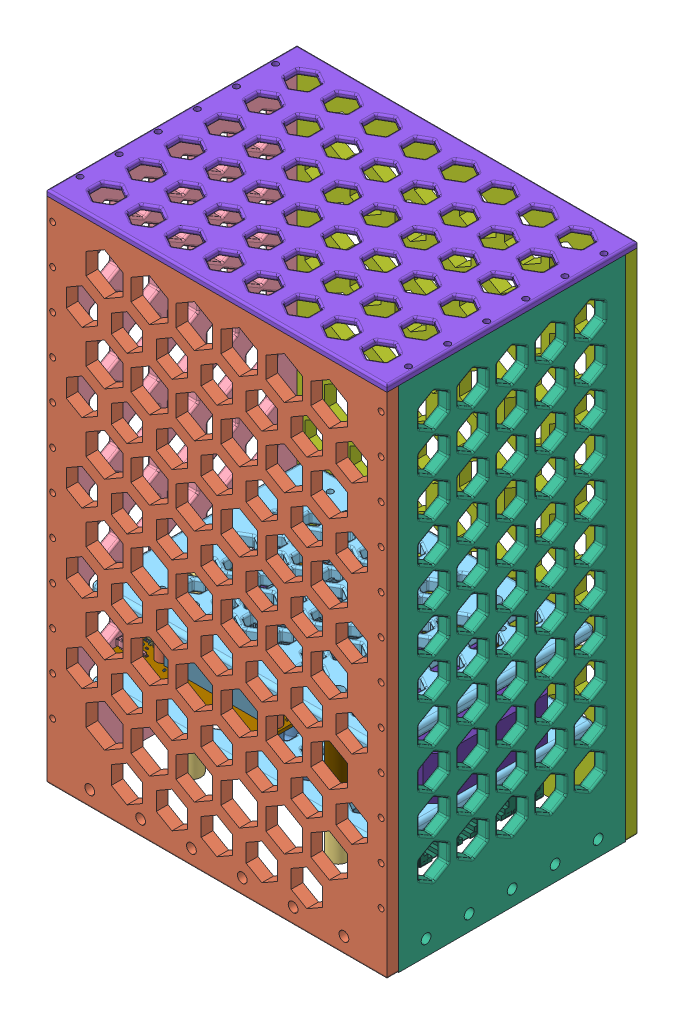
SolidWorks assembly upperbody, configuration 默认. Lengths in mm.
Overall size (174 266.08 128).
496 component instances, 112 part files, 71 mates.
Components (placement in the parent):
- battery-1: battery [默认] at (3.2915 206.5588 214.1011) x (-1 0 0) z (0 -1 0) size (140 115 140)
- imu-1: imu [默认] at (5.7743 27.9888 133.0371) x (0 0 -1) z (0 1 0) size (79.76 40 69.46)
- front-1: front [默认] at (4.5084 194.9888 220) size (174 260 6)
- M8螺柱-1: M8螺柱 [默认] at (42.5084 62.9888 122) size (10 25 10)
- M8螺柱-2: M8螺柱 [默认] at (42.5084 62.9888 202) x (0.721666 0 -0.692241) z (0.692241 0 0.721666) size (10 25 10)
- M8螺柱-3: M8螺柱 [默认] at (-32.4916 62.9888 122) x (0.928948 0 -0.370211) z (0.370211 0 0.928948) size (10 25 10)
- M8螺柱-4: M8螺柱 [默认] at (-32.4916 62.9888 202) x (0.697956 0 -0.71614) z (0.71614 0 0.697956) size (10 25 10)
- left-1: left [默认] at (-82.4916 204.9888 162) x (0 0 -1) z (1 0 0) size (116 260 6)
- ctrlbox-2: ctrlbox [默认] at (5.0084 87.9888 162) size (148 6 110)
- right-1: right [默认] at (91.5084 204.9888 162) x (0 0 1) z (-1 0 0) size (116 260 6)
- back-2: back [默认] at (4.5084 194.9888 98) size (174 260 6)
- top-1: top [默认] at (4.5084 304.9888 162) size (174 6.16 128)
- jetsonnano-1: jetsonnano [默认] at (-39.9804 116.3688 223.5192) x (0 0 1) z (0 1 0) size (100.18 80.53 31.78)
  - 675_13541_batuu_dev_kit_top_ass_asm.stp-1: 675_13541_batuu_dev_kit_top_ass_asm.stp [Default] at (-107.5192 -7.5112 -12.38) size (100.18 80.53 31.78)
    - 642-13541_BATUU_SYS_BOM_ASM.stp-1: 642-13541_BATUU_SYS_BOM_ASM.stp [Default] at origin size (100.18 80.53 21.55)
      - 600-13542-BASE-A02_ASM.stp-1: 600-13542-BASE-A02_ASM.stp [Default] at origin size (100.18 80.53 21.55)
        - 600-13542-BASE-A02.stp-1: 600-13542-BASE-A02.stp [Default] at origin size (100 79 1.57)
        - 064-0473-000_1.stp-1: 064-0473-000_1.stp [Default] at (2.055 -14.41 1.57) size (11.16 8.51 5.94)
        - LOGO_SILK_180_I560.stp-1: LOGO_SILK_180_I560.stp [Default] at (2.088 17.507 0) x (0 1 0) z (0 0 -1) size (14.3 1.27 0.05)
        - LOGO_SILK_POSTAL_ADDRESS.stp-1: LOGO_SILK_POSTAL_ADDRESS.stp [Default] at (3.985 7.597 0) x (0 1 0) z (0 0 -1) size (18.11 2.17 0.05)
        - LS_ICES_I0925X0040_CLASS_B.stp-1: LS_ICES_I0925X0040_CLASS_B.stp [Default] at (0.822 15.645 0) x (0 1 0) z (0 0 -1) size (17.94 1.42 0.03)
        - LOGO_SILK_P3542.stp-1: LOGO_SILK_P3542.stp [Default] at (-1.446 36.987 0) x (0 1 0) z (0 0 -1) size (6.18 1.16 0.01)
        - LOGO_SILK_ROHS_I0300X0153.stp-1: LOGO_SILK_ROHS_I0300X0153.stp [Default] at (0.509 33.093 0) x (0 1 0) z (0 0 -1) size (7.55 3.9 0.05)
        - LOGO_SILK_NVIDIA_I0400X0240.stp-1: LOGO_SILK_NVIDIA_I0400X0240.stp [Default] at (10.037 11.31 0) x (0 1 0) z (0 0 -1) size (7.63 5.72 0.1)
        - 115-1921-000_3.stp-1: 115-1921-000_3.stp [Default] at (71 38 1.57) x (0 -1 0) z (0 0 1) size (5 4 1.01)
        - 115-1921-000_3.stp-2: 115-1921-000_3.stp [Default] at (71 46.5 1.57) x (0 -1 0) z (0 0 1) size (5 4 1.01)
        - 115-1921-000_3.stp-3: 115-1921-000_3.stp [Default] at (71 29.5 1.57) x (0 -1 0) z (0 0 1) size (5 4 1.01)
        - LS_CTUVUS_0500X0500_SIMPLE.stp-1: LS_CTUVUS_0500X0500_SIMPLE.stp [Default] at (49.36 31.942 0) x (-1 0 0) z (0 0 -1) size (5.04 5.01 0.05)
        - LOGO_SILK_UKRAINE_0500X0500.stp-1: LOGO_SILK_UKRAINE_0500X0500.stp [Default] at (41 32.494 0) x (-1 0 0) z (0 0 -1) size (4.37 5.01 0.05)
        - LOGO_SILK_SAA_1206X0540.stp-1: LOGO_SILK_SAA_1206X0540.stp [Default] at (44.276 41.966 0) x (-1 0 0) z (0 0 -1) size (12.08 8.03 0.06)
        - 064-0476-000_1.stp-1: 064-0476-000_1.stp [Default] at (55.6 -9.269 1.57) size (14.86 17.99 18.47)
        - 064-0472-000_1.stp-1: 064-0472-000_1.stp [Default] at (88 -14.3 1.57) size (8.8 6.34 3.46)
        - 0402_SHUNT_NO.stp-1: 0402_SHUNT_NO.stp [Default] at (57.444 37.6 1.57) size (1.51 0.51 0.03)
        - 0402_SHUNT_NO.stp-2: 0402_SHUNT_NO.stp [Default] at (55.15 36.025 1.57) x (0 1 0) z (0 0 1) size (1.51 0.51 0.03)
        - 0402_SHUNT_NO.stp-3: 0402_SHUNT_NO.stp [Default] at (55.15 33.762 1.57) x (0 -1 0) z (0 0 1) size (1.51 0.51 0.03)
        - 0402_SHORT.stp-1: 0402_SHORT.stp [Default] at (57.6 38.53 1.57) size (1.51 0.51 1)
        - 0402_SHORT.stp-2: 0402_SHORT.stp [Default] at (53.708 35.675 1.57) x (-1 0 0) z (0 0 1) size (1.51 0.51 1)
        - 0402_SHORT.stp-3: 0402_SHORT.stp [Default] at (53.708 34.112 1.57) x (-1 0 0) z (0 0 1) size (1.51 0.51 1)
        - 0402_SHORT.stp-4: 0402_SHORT.stp [Default] at (60.9 37.1 1.57) x (0 -1 0) z (0 0 1) size (1.51 0.51 1)
        - 064-0474-000_1.stp-1: 064-0474-000_1.stp [Default] at (38.6 -9.759 1.57) size (14.81 17.11 9.91)
        - 085-0347-000_1.stp-1: 085-0347-000_1.stp [Default] at (31.173 31.804 1.57) x (0 -1 0) z (0 0 1) size (3.6 2.9 0.81)
        - 115-2844-000_1.stp-1: 115-2844-000_1.stp [Default] at (39.89 33.254 1.57) x (0 1 0) z (0 0 1) size (5.01 7.06 1.76)
        - 074-0259-000_1.stp-1: 074-0259-000_1.stp [Default] at (19.751 -12.06 1.57) x (0 1 0) z (0 0 1) size (13.02 16.16 8.1)
        - 106-0078-000_1.stp-1: 106-0078-000_1.stp [Default] at (4.864 -6.11 1.57) size (6.08 4.44 1.61)
        - LOGO_SILK_EAC_050X050.stp-1: LOGO_SILK_EAC_050X050.stp [Default] at (28.157 35.506 0) x (-1 0 0) z (0 0 -1) size (5 5 0.05)
        - LOGO_LABEL_PPID_0180X0050.stp-1: LOGO_LABEL_PPID_0180X0050.stp [Default] at (49.45 19.35 0) x (-1 0 0) z (0 0 -1) size (18 5 0.15)
        - 074-0221-000_3.stp-1: 074-0221-000_3.stp [Default] at (86 29 1.57) x (0 1 0) z (0 0 1) size (51.01 5.29 12.01)
        - 080-1656-000_3.stp-1: 080-1656-000_3.stp [Default] at (44 16.6 1.57) x (-1 0 0) z (0 0 1) size (77.5 26.11 9.91)
        - 080-1669-000_2.stp-1: 080-1669-000_2.stp [Default] at (0.2 29 1.57) x (0 -1 0) z (0 0 1) size (22.61 5.4 8.01)
        - 064-0400-000_1.stp-1: 064-0400-000_1.stp [Default] at (67.5 7.785 1.57) size (10.42 6.06 13.91)
        - 220-0146-000_2.stp-1: 220-0146-000_2.stp [Default] at (59.96 55.2 0) x (-1 0 0) z (0 0 -1) size (19.53 12.33 3.44)
        - 074-0239-000_1.stp-1: 074-0239-000_1.stp [Default] at (31.71 54.5 1.57) x (-1 0 0) z (0 0 1) size (30.59 10.8 5.76)
        - 0603_H100.stp-1: 0603_H100.stp [Default] at (34.617 32.966 1.57) x (0 1 0) z (0 0 1) size (1.81 1.01 1.01)
        - 0603_H100.stp-2: 0603_H100.stp [Default] at (33.893 7.175 1.57) x (-1 0 0) z (0 0 1) size (1.81 1.01 1.01)
        - 0603_H100.stp-3: 0603_H100.stp [Default] at (20.2 35 1.57) x (-1 0 0) z (0 0 1) size (1.81 1.01 1.01)
        - 0603_H100.stp-4: 0603_H100.stp [Default] at (20.2 33.55 1.57) x (-1 0 0) z (0 0 1) size (1.81 1.01 1.01)
        - 0603_H100.stp-5: 0603_H100.stp [Default] at (13.895 41.85 1.57) x (-1 0 0) z (0 0 1) size (1.81 1.01 1.01)
        - 0603_H100.stp-6: 0603_H100.stp [Default] at (7.3 3.117 1.57) size (1.81 1.01 1.01)
        - 0603_H100.stp-7: 0603_H100.stp [Default] at (11.03 6.374 1.57) x (0 1 0) z (0 0 1) size (1.81 1.01 1.01)
        - 0603_H060.stp-1: 0603_H060.stp [Default] at (63.195 1.13 1.57) size (1.81 1.02 0.61)
        - 0603_H060.stp-2: 0603_H060.stp [Default] at (82.541 -6.821 1.57) x (-1 0 0) z (0 0 1) size (1.81 1.02 0.61)
        - 0603_H060.stp-3: 0603_H060.stp [Default] at (82.541 -9.047 1.57) x (-1 0 0) z (0 0 1) size (1.81 1.02 0.61)
        - FID_40_80SM.stp-1: FID_40_80SM.stp [Default] at (80.7 59.5 1.57) size (2.29 2.29 0.05)
        - FID_40_80SM.stp-2: FID_40_80SM.stp [Default] at (7.943 54.544 1.57) size (2.29 2.29 0.05)
        - FID_40_80SM.stp-3: FID_40_80SM.stp [Default] at (93.132 -0.325 1.57) size (2.29 2.29 0.05)
        - FID_40_80SM.stp-4: FID_40_80SM.stp [Default] at (9.9 22.4 0) x (-1 0 0) z (0 0 -1) size (2.29 2.29 0.05)
        - FID_40_80SM.stp-5: FID_40_80SM.stp [Default] at (80.7 59.5 0) x (-1 0 0) z (0 0 -1) size (2.29 2.29 0.05)
        - FID_40_80SM.stp-6: FID_40_80SM.stp [Default] at (3.95 -6.475 0) x (-1 0 0) z (0 0 -1) size (2.29 2.29 0.05)
        - LOGO_SILK_ROHS_D050_CHINA.stp-1: LOGO_SILK_ROHS_D050_CHINA.stp [Default] at (35.305 32.341 0) x (-1 0 0) z (0 0 -1) size (5.62 4.99 0.05)
        - LOGO_SILK_WEEE_0485X0683.stp-1: LOGO_SILK_WEEE_0485X0683.stp [Default] at (28.183 29 0) x (-1 0 0) z (0 0 -1) size (4.85 6.82 0.05)
        - LOGO_SILK_VCCI_I0300X0225.stp-1: LOGO_SILK_VCCI_I0300X0225.stp [Default] at (55.897 33.25 0) x (-1 0 0) z (0 0 -1) size (8.32 6.14 0.05)
        - LOGO_SILK_RCM_040X030.stp-1: LOGO_SILK_RCM_040X030.stp [Default] at (57.832 27.06 0) x (-1 0 0) z (0 0 -1) size (4.05 3 0.05)
        - LOGO_SILK_BSMI_I0138H.stp-1: LOGO_SILK_BSMI_I0138H.stp [Default] at (52.892 27.23 0) x (-1 0 0) z (0 0 -1) size (8.8 3.76 0.05)
        - LOGO_SILK_HF_I0185X0120.stp-1: LOGO_SILK_HF_I0185X0120.stp [Default] at (37.6 25.2 0) x (-1 0 0) z (0 0 -1) size (4.83 3.17 0.07)
        - 090-0243-000_1.stp-1: 090-0243-000_1.stp [Default] at (88.606 -9.875 1.57) size (1.41 0.71 0.46)
        - 090-0243-000_1.stp-2: 090-0243-000_1.stp [Default] at (86.685 -9.875 1.57) x (-1 0 0) z (0 0 1) size (1.41 0.71 0.46)
        - 090-0243-000_1.stp-3: 090-0243-000_1.stp [Default] at (43.22 0.665 1.57) size (1.41 0.71 0.46)
        - 090-0243-000_1.stp-4: 090-0243-000_1.stp [Default] at (41.15 0.665 1.57) x (-1 0 0) z (0 0 1) size (1.41 0.71 0.46)
        - 090-0243-000_1.stp-5: 090-0243-000_1.stp [Default] at (11.85 27.85 1.57) size (1.41 0.71 0.46)
        - 090-0243-000_1.stp-6: 090-0243-000_1.stp [Default] at (12.358 6.374 1.57) x (0 1 0) z (0 0 1) size (1.41 0.71 0.46)
        - 090-0243-000_1.stp-7: 090-0243-000_1.stp [Default] at (19.35 -1.5 1.57) size (1.41 0.71 0.46)
        - 090-0243-000_1.stp-8: 090-0243-000_1.stp [Default] at (17.358 -1.5 1.57) size (1.41 0.71 0.46)
        - 090-0243-000_1.stp-9: 090-0243-000_1.stp [Default] at (15.308 -1.5 1.57) x (-1 0 0) z (0 0 1) size (1.41 0.71 0.46)
        - 090-0243-000_1.stp-10: 090-0243-000_1.stp [Default] at (13.064 -4.054 1.57) x (-1 0 0) z (0 0 1) size (1.41 0.71 0.46)
        - 090-0243-000_1.stp-11: 090-0243-000_1.stp [Default] at (3.491 18.432 1.57) x (0 -1 0) z (0 0 1) size (1.41 0.71 0.46)
        - 090-0243-000_1.stp-12: 090-0243-000_1.stp [Default] at (5.016 18.432 1.57) x (0 -1 0) z (0 0 1) size (1.41 0.71 0.46)
        - 090-0243-000_1.stp-13: 090-0243-000_1.stp [Default] at (11.85 23.6 1.57) size (1.41 0.71 0.46)
        - 090-0243-000_1.stp-14: 090-0243-000_1.stp [Default] at (11.85 25.25 1.57) size (1.41 0.71 0.46)
        - 090-0243-000_1.stp-15: 090-0243-000_1.stp [Default] at (11.85 26.5 1.57) size (1.41 0.71 0.46)
        - 091-0023-000_1.stp-1: 091-0023-000_1.stp [Default] at (17.098 5.642 1.57) size (2.21 2.51 1.11)
        - 115-2747-000_1.stp-1: 115-2747-000_1.stp [Default] at (11.957 32.276 1.57) x (0 1 0) z (0 0 1) size (2.21 2.88 1.11)
        - 115-0742-000_2.stp-1: 115-0742-000_2.stp [Default] at (5.725 44.6 1.57) size (2.21 2.88 1.11)
        - 115-1821-000_1.stp-1: 115-1821-000_1.stp [Default] at (12.1 48.825 1.57) x (0 -1 0) z (0 0 1) size (2.21 2.88 1.11)
        - 115-1821-000_1.stp-2: 115-1821-000_1.stp [Default] at (8.55 44.6 1.57) x (-1 0 0) z (0 0 1) size (2.21 2.88 1.11)
        - 115-0138-000_1.stp-1: 115-0138-000_1.stp [Default] at (59.536 5.825 1.57) x (-1 0 0) z (0 0 1) size (2.21 2.88 1.11)
        - 115-0742-000_2.stp-2: 115-0742-000_2.stp [Default] at (11.3 44.6 1.57) x (-1 0 0) z (0 0 1) size (2.21 2.88 1.11)
        - 315-1048-000_1.stp-1: 315-1048-000_1.stp [Default] at (7.151 6.724 1.57) x (0 1 0) z (0 0 1) size (3.11 3.58 1.46)
        - 315-1014-000_1.stp-1: 315-1014-000_1.stp [Default] at (36.977 7.376 1.57) size (3.11 3.58 1.46)
        - 315-0620-000_1.stp-1: 315-0620-000_1.stp [Default] at (53.589 41.71 1.57) x (0 -1 0) z (0 0 1) size (3.11 3.58 1.11)
        - LOGO_SILK_CE_I0175X0160.stp-1: LOGO_SILK_CE_I0175X0160.stp [Default] at (41.179 26.706 0) x (-1 0 0) z (0 0 -1) size (4.55 3.29 0.05)
        - 090-0231-000_1.stp-1: 090-0231-000_1.stp [Default] at (56.393 1.13 1.57) x (-1 0 0) z (0 0 1) size (2.61 1.55 0.56)
        - 090-0231-000_1.stp-2: 090-0231-000_1.stp [Default] at (25.625 -1.95 1.57) x (-1 0 0) z (0 0 1) size (2.61 1.55 0.56)
        - 090-0231-000_1.stp-3: 090-0231-000_1.stp [Default] at (21.95 -1.95 1.57) size (2.61 1.55 0.56)
        - 090-0231-000_1.stp-4: 090-0231-000_1.stp [Default] at (38.6 0.417 1.57) size (2.61 1.55 0.56)
        - 0402_H040.stp-1: 0402_H040.stp [Default] at (61.419 6.962 1.57) x (0 1 0) z (0 0 1) size (1.2 0.61 0.41)
        - 0402_H060.stp-1: 0402_H060.stp [Default] at (3.646 48.98 1.57) x (0 -1 0) z (0 0 1) size (1.11 0.61 0.61)
        - 0402_H060.stp-2: 0402_H060.stp [Default] at (82.141 -12.349 1.57) x (-1 0 0) z (0 0 1) size (1.11 0.61 0.61)
        - 0402_H060.stp-3: 0402_H060.stp [Default] at (85.011 -10.767 1.57) x (-1 0 0) z (0 0 1) size (1.11 0.61 0.61)
        - 0402_H040.stp-2: 0402_H040.stp [Default] at (57.017 6.2 1.57) x (0 1 0) z (0 0 1) size (1.2 0.61 0.41)
        - 0402_H060.stp-4: 0402_H060.stp [Default] at (50.674 42.15 1.57) x (0 -1 0) z (0 0 1) size (1.11 0.61 0.61)
        - 0402_H060.stp-5: 0402_H060.stp [Default] at (56.489 42.038 1.57) x (0 -1 0) z (0 0 1) size (1.11 0.61 0.61)
        - 0402_H060.stp-6: 0402_H060.stp [Default] at (9.475 49.55 1.57) x (0 1 0) z (0 0 1) size (1.11 0.61 0.61)
        - 0402_H040.stp-3: 0402_H040.stp [Default] at (35.099 35.617 1.57) size (1.2 0.61 0.41)
        - 0402_H040.stp-4: 0402_H040.stp [Default] at (37.596 37.35 1.57) x (-1 0 0) z (0 0 1) size (1.2 0.61 0.41)
        - 0402_H040.stp-5: 0402_H040.stp [Default] at (85.653 -8.168 1.57) x (0 1 0) z (0 0 1) size (1.2 0.61 0.41)
        - 0402_H060.stp-7: 0402_H060.stp [Default] at (33.493 30.304 1.57) x (0 1 0) z (0 0 1) size (1.11 0.61 0.61)
        - 0402_H060.stp-8: 0402_H060.stp [Default] at (33.493 32.251 1.57) x (0 1 0) z (0 0 1) size (1.11 0.61 0.61)
        - 0402_H060.stp-9: 0402_H060.stp [Default] at (35.099 34.667 1.57) x (-1 0 0) z (0 0 1) size (1.11 0.61 0.61)
        - 0402_H060.stp-10: 0402_H060.stp [Default] at (33.45 36.567 1.57) x (-1 0 0) z (0 0 1) size (1.11 0.61 0.61)
        - 0402_H060.stp-11: 0402_H060.stp [Default] at (33.45 35.617 1.57) x (-1 0 0) z (0 0 1) size (1.11 0.61 0.61)
        - 0402_H040.stp-6: 0402_H040.stp [Default] at (14.693 -3.538 1.57) x (0 -1 0) z (0 0 1) size (1.2 0.61 0.41)
        - 0402_H060.stp-12: 0402_H060.stp [Default] at (50.945 26.269 1.57) size (1.11 0.61 0.61)
        - 0402_H060.stp-13: 0402_H060.stp [Default] at (53.281 0.53 1.57) size (1.11 0.61 0.61)
        - 0402_H060.stp-14: 0402_H060.stp [Default] at (30.208 -2.121 1.57) x (-1 0 0) z (0 0 1) size (1.11 0.61 0.61)
        - 0402_H040.stp-7: 0402_H040.stp [Default] at (5.44 41.7 1.57) x (-1 0 0) z (0 0 1) size (1.2 0.61 0.41)
        - 0402_H060.stp-15: 0402_H060.stp [Default] at (21.109 6.878 1.57) x (0 -1 0) z (0 0 1) size (1.11 0.61 0.61)
        - 0402_H040.stp-8: 0402_H040.stp [Default] at (12.1 46.85 1.57) size (1.2 0.61 0.41)
        - 0402_H040.stp-9: 0402_H040.stp [Default] at (89.1 -4.75 1.57) x (-1 0 0) z (0 0 1) size (1.2 0.61 0.41)
        - 0402_H040.stp-10: 0402_H040.stp [Default] at (73.778 10.336 1.57) x (-1 0 0) z (0 0 1) size (1.2 0.61 0.41)
        - 0402_H040.stp-11: 0402_H040.stp [Default] at (16.95 -0.35 1.57) x (-1 0 0) z (0 0 1) size (1.2 0.61 0.41)
        - 0402_H040.stp-12: 0402_H040.stp [Default] at (15.333 -0.35 1.57) size (1.2 0.61 0.41)
        - 0402_H040.stp-13: 0402_H040.stp [Default] at (18.957 4.734 1.57) x (0 1 0) z (0 0 1) size (1.2 0.61 0.41)
        - 0402_H040.stp-14: 0402_H040.stp [Default] at (14.912 7.235 1.57) x (-1 0 0) z (0 0 1) size (1.2 0.61 0.41)
        - 0402_H040.stp-15: 0402_H040.stp [Default] at (31.504 6.574 1.57) x (-1 0 0) z (0 0 1) size (1.2 0.61 0.41)
        - 0402_H040.stp-16: 0402_H040.stp [Default] at (29.859 6.574 1.57) size (1.2 0.61 0.41)
        - 0402_H060.stp-16: 0402_H060.stp [Default] at (38.505 2.843 1.57) x (0 -1 0) z (0 0 1) size (1.11 0.61 0.61)
        - 0402_H060.stp-17: 0402_H060.stp [Default] at (34.05 8.75 1.57) x (-1 0 0) z (0 0 1) size (1.11 0.61 0.61)
        - 0402_H060.stp-18: 0402_H060.stp [Default] at (37.594 2.843 1.57) x (0 -1 0) z (0 0 1) size (1.11 0.61 0.61)
        - 0402_H040.stp-17: 0402_H040.stp [Default] at (44.5 9.25 1.57) size (1.2 0.61 0.41)
        - 0402_H040.stp-18: 0402_H040.stp [Default] at (6.98 47.3 1.57) size (1.2 0.61 0.41)
        - 0402_H040.stp-19: 0402_H040.stp [Default] at (82.141 -11.445 1.57) x (-1 0 0) z (0 0 1) size (1.2 0.61 0.41)
        - 0402_H040.stp-20: 0402_H040.stp [Default] at (63.62 -11.35 1.57) x (0 -1 0) z (0 0 1) size (1.2 0.61 0.41)
        - 0402_H060.stp-19: 0402_H060.stp [Default] at (39.409 2.843 1.57) x (0 -1 0) z (0 0 1) size (1.11 0.61 0.61)
        - 0402_H060.stp-20: 0402_H060.stp [Default] at (40.35 2.843 1.57) x (0 -1 0) z (0 0 1) size (1.11 0.61 0.61)
        - 0402_H060.stp-21: 0402_H060.stp [Default] at (4.425 -9.55 1.57) size (1.11 0.61 0.61)
        - 0402_H060.stp-22: 0402_H060.stp [Default] at (26.7 47 1.57) size (1.11 0.61 0.61)
        - 0402_H070.stp-1: 0402_H070.stp [Default] at (20.2 36.2 1.57) x (-1 0 0) z (0 0 1) size (1.11 0.61 0.71)
        - 0402_H060.stp-23: 0402_H060.stp [Default] at (5.44 40.55 1.57) size (1.11 0.61 0.61)
        - 0402_H060.stp-24: 0402_H060.stp [Default] at (57.017 7.825 1.57) x (0 1 0) z (0 0 1) size (1.11 0.61 0.61)
        - 0402_H060.stp-25: 0402_H060.stp [Default] at (73.65 4 1.57) size (1.11 0.61 0.61)
        - 0402_H060.stp-26: 0402_H060.stp [Default] at (82.141 -10.442 1.57) size (1.11 0.61 0.61)
        - 0402_H060.stp-27: 0402_H060.stp [Default] at (63.37 3.231 1.57) size (1.11 0.61 0.61)
        - 0402_H060.stp-28: 0402_H060.stp [Default] at (6.652 4.356 1.57) size (1.11 0.61 0.61)
        - 0402_H060.stp-29: 0402_H060.stp [Default] at (24.377 6.917 1.57) x (0 -1 0) z (0 0 1) size (1.11 0.61 0.61)
        - 0402_H060.stp-30: 0402_H060.stp [Default] at (27.693 6.896 1.57) x (0 -1 0) z (0 0 1) size (1.11 0.61 0.61)
        - 0402_H060.stp-31: 0402_H060.stp [Default] at (30.18 7.846 1.57) x (0 -1 0) z (0 0 1) size (1.11 0.61 0.61)
        - 0402_H060.stp-32: 0402_H060.stp [Default] at (22.059 6.878 1.57) x (0 -1 0) z (0 0 1) size (1.11 0.61 0.61)
        - 0402_H060.stp-33: 0402_H060.stp [Default] at (25.377 6.917 1.57) x (0 -1 0) z (0 0 1) size (1.11 0.61 0.61)
        - 0402_H060.stp-34: 0402_H060.stp [Default] at (28.602 6.896 1.57) x (0 -1 0) z (0 0 1) size (1.11 0.61 0.61)
        - 0402_H060.stp-35: 0402_H060.stp [Default] at (31.154 7.846 1.57) x (0 -1 0) z (0 0 1) size (1.11 0.61 0.61)
        - 0402_H060.stp-36: 0402_H060.stp [Default] at (15.954 -4.338 1.57) size (1.11 0.61 0.61)
        - 0402_H060.stp-37: 0402_H060.stp [Default] at (13.93 5.406 1.57) x (-1 0 0) z (0 0 1) size (1.11 0.61 0.61)
        - 0402_H060.stp-38: 0402_H060.stp [Default] at (15.95 -2.95 1.57) x (-1 0 0) z (0 0 1) size (1.11 0.61 0.61)
        - 0402_H060.stp-39: 0402_H060.stp [Default] at (19.2 -2.95 1.57) size (1.11 0.61 0.61)
        - 0402_H060.stp-40: 0402_H060.stp [Default] at (17.551 -2.95 1.57) size (1.11 0.61 0.61)
        - 0402_H060.stp-41: 0402_H060.stp [Default] at (13.064 -2.95 1.57) x (-1 0 0) z (0 0 1) size (1.11 0.61 0.61)
        - 0402_H060.stp-42: 0402_H060.stp [Default] at (2.85 37.55 1.57) x (0 1 0) z (0 0 1) size (1.11 0.61 0.61)
        - 0402_H060.stp-43: 0402_H060.stp [Default] at (68.15 40.157 1.57) x (0 1 0) z (0 0 1) size (1.11 0.61 0.61)
        - 0402_H060.stp-44: 0402_H060.stp [Default] at (73.85 40.157 1.57) x (0 1 0) z (0 0 1) size (1.11 0.61 0.61)
        - 0402_H060.stp-45: 0402_H060.stp [Default] at (90.95 6.1 1.57) size (1.11 0.61 0.61)
        - 0402_H060.stp-46: 0402_H060.stp [Default] at (68.167 49.132 1.57) x (0 1 0) z (0 0 1) size (1.11 0.61 0.61)
        - 0402_H060.stp-47: 0402_H060.stp [Default] at (59.769 3.59 1.57) x (-1 0 0) z (0 0 1) size (1.11 0.61 0.61)
        - 0402_H060.stp-48: 0402_H060.stp [Default] at (73.85 48.646 1.57) x (0 1 0) z (0 0 1) size (1.11 0.61 0.61)
        - 0402_H060.stp-49: 0402_H060.stp [Default] at (68.15 31.652 1.57) x (0 1 0) z (0 0 1) size (1.11 0.61 0.61)
        - 0402_H060.stp-50: 0402_H060.stp [Default] at (73.85 31.66 1.57) x (0 1 0) z (0 0 1) size (1.11 0.61 0.61)
        - 0402_H060.stp-51: 0402_H060.stp [Default] at (39.15 45.85 1.57) x (-1 0 0) z (0 0 1) size (1.11 0.61 0.61)
        - 0402_H060.stp-52: 0402_H060.stp [Default] at (39.15 46.878 1.57) x (-1 0 0) z (0 0 1) size (1.11 0.61 0.61)
        - 0402_H060.stp-53: 0402_H060.stp [Default] at (73.778 8.083 1.57) x (0 -1 0) z (0 0 1) size (1.11 0.61 0.61)
        - 0402_H060.stp-54: 0402_H060.stp [Default] at (27.5 49.75 1.57) x (-1 0 0) z (0 0 1) size (1.11 0.61 0.61)
        - 0402_H060.stp-55: 0402_H060.stp [Default] at (59.5 37.1 1.57) x (-1 0 0) z (0 0 1) size (1.11 0.61 0.61)
        - 0402_H040.stp-21: 0402_H040.stp [Default] at (14.621 0.778 1.57) x (-1 0 0) z (0 0 1) size (1.2 0.61 0.41)
        - 0402_H040.stp-22: 0402_H040.stp [Default] at (14.887 6.314 1.57) size (1.2 0.61 0.41)
        - 0402_H040.stp-23: 0402_H040.stp [Default] at (13.555 7.126 1.57) x (0 -1 0) z (0 0 1) size (1.2 0.61 0.41)
        - 0402_H040.stp-24: 0402_H040.stp [Default] at (12.661 0.478 1.57) x (0 1 0) z (0 0 1) size (1.2 0.61 0.41)
        - 0402_H040.stp-25: 0402_H040.stp [Default] at (53.55 23.2 1.57) x (0 1 0) z (0 0 1) size (1.2 0.61 0.41)
        - 0402_H040.stp-26: 0402_H040.stp [Default] at (57.842 9.9 1.57) x (0 1 0) z (0 0 1) size (1.2 0.61 0.41)
        - 0402_H040.stp-27: 0402_H040.stp [Default] at (58.75 9.9 1.57) x (0 1 0) z (0 0 1) size (1.2 0.61 0.41)
        - 0402_H040.stp-28: 0402_H040.stp [Default] at (60.45 32.794 1.57) x (0 1 0) z (0 0 1) size (1.2 0.61 0.41)
        - 0402_H040.stp-29: 0402_H040.stp [Default] at (61.787 35.7 1.57) x (0 -1 0) z (0 0 1) size (1.2 0.61 0.41)
        - 0402_H040.stp-30: 0402_H040.stp [Default] at (60.15 9.9 1.57) x (0 1 0) z (0 0 1) size (1.2 0.61 0.41)
        - 0402_H040.stp-31: 0402_H040.stp [Default] at (3.646 43.6 1.57) x (0 1 0) z (0 0 1) size (1.2 0.61 0.41)
        - 0402_H040.stp-32: 0402_H040.stp [Default] at (61.075 9.9 1.57) x (0 1 0) z (0 0 1) size (1.2 0.61 0.41)
        - 0402_H040.stp-33: 0402_H040.stp [Default] at (13 36.398 1.57) x (0 -1 0) z (0 0 1) size (1.2 0.61 0.41)
        - 0402_H040.stp-34: 0402_H040.stp [Default] at (11.693 36.398 1.57) x (0 -1 0) z (0 0 1) size (1.2 0.61 0.41)
        - 0402_H040.stp-35: 0402_H040.stp [Default] at (-1.925 -7.511 1.57) x (-1 0 0) z (0 0 1) size (1.2 0.61 0.41)
        - 0402_H040.stp-36: 0402_H040.stp [Default] at (-1.925 -6.588 1.57) x (-1 0 0) z (0 0 1) size (1.2 0.61 0.41)
        - 0402_H040.stp-37: 0402_H040.stp [Default] at (10.28 1.69 1.57) x (0 1 0) z (0 0 1) size (1.2 0.61 0.41)
        - 0402_H040.stp-38: 0402_H040.stp [Default] at (11.49 -3.788 1.57) x (0 -1 0) z (0 0 1) size (1.2 0.61 0.41)
        - 0402_H040.stp-39: 0402_H040.stp [Default] at (35.418 10.679 1.57) x (0 1 0) z (0 0 1) size (1.2 0.61 0.41)
        - 0402_H040.stp-40: 0402_H040.stp [Default] at (41.66 2.685 1.57) x (0 -1 0) z (0 0 1) size (1.2 0.61 0.41)
        - 0402_H040.stp-41: 0402_H040.stp [Default] at (42.61 2.685 1.57) x (0 -1 0) z (0 0 1) size (1.2 0.61 0.41)
        - 0402_H040.stp-42: 0402_H040.stp [Default] at (50.15 1.275 1.57) size (1.2 0.61 0.41)
        - 0402_H040.stp-43: 0402_H040.stp [Default] at (50.15 2.225 1.57) size (1.2 0.61 0.41)
        - 0402_H040.stp-44: 0402_H040.stp [Default] at (50.173 3.305 1.57) size (1.2 0.61 0.41)
        - 0402_H040.stp-45: 0402_H040.stp [Default] at (50.173 4.255 1.57) size (1.2 0.61 0.41)
        - 0402_H040.stp-46: 0402_H040.stp [Default] at (53.589 39.034 1.57) x (-1 0 0) z (0 0 1) size (1.2 0.61 0.41)
        - 0402_H040.stp-47: 0402_H040.stp [Default] at (24.4 47.25 1.57) x (0 1 0) z (0 0 1) size (1.2 0.61 0.41)
        - 0402_H040.stp-48: 0402_H040.stp [Default] at (26.7 47.9 1.57) size (1.2 0.61 0.41)
        - 0402_H040.stp-49: 0402_H040.stp [Default] at (25.9 48.85 1.57) x (-1 0 0) z (0 0 1) size (1.2 0.61 0.41)
        - 0402_H040.stp-50: 0402_H040.stp [Default] at (7.975 41.7 1.57) x (-1 0 0) z (0 0 1) size (1.2 0.61 0.41)
        - 0402_H040.stp-51: 0402_H040.stp [Default] at (14.095 40.55 1.57) size (1.2 0.61 0.41)
        - 0402_H040.stp-52: 0402_H040.stp [Default] at (61.419 5.325 1.57) x (0 1 0) z (0 0 1) size (1.2 0.61 0.41)
        - 0402_H040.stp-53: 0402_H040.stp [Default] at (11.3 42.2 1.57) x (-1 0 0) z (0 0 1) size (1.2 0.61 0.41)
        - 0402_H040.stp-54: 0402_H040.stp [Default] at (5.375 47.3 1.57) size (1.2 0.61 0.41)
        - 0402_H040.stp-55: 0402_H040.stp [Default] at (82.541 -5.697 1.57) x (-1 0 0) z (0 0 1) size (1.2 0.61 0.41)
        - 0402_H040.stp-56: 0402_H040.stp [Default] at (82.141 -7.946 1.57) x (-1 0 0) z (0 0 1) size (1.2 0.61 0.41)
        - 0402_H040.stp-57: 0402_H040.stp [Default] at (63.37 2.26 1.57) size (1.2 0.61 0.41)
        - 0402_H040.stp-58: 0402_H040.stp [Default] at (52.6 23.2 1.57) x (0 1 0) z (0 0 1) size (1.2 0.61 0.41)
        - 0402_H040.stp-59: 0402_H040.stp [Default] at (15.583 8.9 1.57) x (0 -1 0) z (0 0 1) size (1.2 0.61 0.41)
        - 0402_H040.stp-60: 0402_H040.stp [Default] at (10.426 8.65 1.57) size (1.2 0.61 0.41)
        - 0402_H040.stp-61: 0402_H040.stp [Default] at (20.747 5.624 1.57) size (1.2 0.61 0.41)
        - 0402_H040.stp-62: 0402_H040.stp [Default] at (22.405 5.624 1.57) x (-1 0 0) z (0 0 1) size (1.2 0.61 0.41)
        - 0402_H040.stp-63: 0402_H040.stp [Default] at (24.029 5.624 1.57) size (1.2 0.61 0.41)
        - 0402_H040.stp-64: 0402_H040.stp [Default] at (25.662 5.624 1.57) x (-1 0 0) z (0 0 1) size (1.2 0.61 0.41)
        - 0402_H040.stp-65: 0402_H040.stp [Default] at (27.303 5.624 1.57) size (1.2 0.61 0.41)
        - 0402_H040.stp-66: 0402_H040.stp [Default] at (28.913 5.624 1.57) x (-1 0 0) z (0 0 1) size (1.2 0.61 0.41)
        - 0402_H040.stp-67: 0402_H040.stp [Default] at (20.725 2.15 1.57) x (0 -1 0) z (0 0 1) size (1.2 0.61 0.41)
        - 0402_H040.stp-68: 0402_H040.stp [Default] at (21.675 2.15 1.57) x (0 -1 0) z (0 0 1) size (1.2 0.61 0.41)
        - 0402_H040.stp-69: 0402_H040.stp [Default] at (23.225 2.15 1.57) x (0 -1 0) z (0 0 1) size (1.2 0.61 0.41)
        - 0402_H040.stp-70: 0402_H040.stp [Default] at (24.175 2.15 1.57) x (0 -1 0) z (0 0 1) size (1.2 0.61 0.41)
        - 0402_H040.stp-71: 0402_H040.stp [Default] at (25.725 2.15 1.57) x (0 -1 0) z (0 0 1) size (1.2 0.61 0.41)
        - 0402_H040.stp-72: 0402_H040.stp [Default] at (26.675 2.15 1.57) x (0 -1 0) z (0 0 1) size (1.2 0.61 0.41)
        - 0402_H040.stp-73: 0402_H040.stp [Default] at (28.225 2.15 1.57) x (0 -1 0) z (0 0 1) size (1.2 0.61 0.41)
        - 0402_H040.stp-74: 0402_H040.stp [Default] at (29.175 2.15 1.57) x (0 -1 0) z (0 0 1) size (1.2 0.61 0.41)
        - 0402_H040.stp-75: 0402_H040.stp [Default] at (12.661 -1.2 1.57) x (0 1 0) z (0 0 1) size (1.2 0.61 0.41)
        - 0402_H040.stp-76: 0402_H040.stp [Default] at (71.114 43.15 1.57) x (-1 0 0) z (0 0 1) size (1.2 0.61 0.41)
        - 0402_H040.stp-77: 0402_H040.stp [Default] at (71.522 34.65 1.57) x (-1 0 0) z (0 0 1) size (1.2 0.61 0.41)
        - 0402_H040.stp-78: 0402_H040.stp [Default] at (57.283 28.368 1.57) x (-1 0 0) z (0 0 1) size (1.2 0.61 0.41)
        - 0402_H040.stp-79: 0402_H040.stp [Default] at (43.941 46.958 1.57) x (-1 0 0) z (0 0 1) size (1.2 0.61 0.41)
        - 0402_H040.stp-80: 0402_H040.stp [Default] at (44.719 46.023 1.57) size (1.2 0.61 0.41)
        - 0402_H040.stp-81: 0402_H040.stp [Default] at (54.672 26.901 1.57) x (0 1 0) z (0 0 1) size (1.2 0.61 0.41)
        - 0402_H040.stp-82: 0402_H040.stp [Default] at (63.1 24.2 1.57) x (0 1 0) z (0 0 1) size (1.2 0.61 0.41)
        - 0402_H040.stp-83: 0402_H040.stp [Default] at (40.75 48.3 1.57) size (1.2 0.61 0.41)
        - 0402_H040.stp-84: 0402_H040.stp [Default] at (44.5 10.25 1.57) size (1.2 0.61 0.41)
        - 0402_H040.stp-85: 0402_H040.stp [Default] at (54.5 23.2 1.57) x (0 1 0) z (0 0 1) size (1.2 0.61 0.41)
        - 0402_H040.stp-86: 0402_H040.stp [Default] at (46.176 10.25 1.57) x (-1 0 0) z (0 0 1) size (1.2 0.61 0.41)
        - 0402_H040.stp-87: 0402_H040.stp [Default] at (46.08 48.3 1.57) size (1.2 0.61 0.41)
        - LTPB071C125D045C025P.stp-1: LTPB071C125D045C025P.stp [Default] at (61.144 33.25 0) x (0 -1 0) z (0 0 -1) size (0.71 0.71 0.08)
        - LTPB071C125D045C025P.stp-2: LTPB071C125D045C025P.stp [Default] at (61.144 34.6 0) x (0 -1 0) z (0 0 -1) size (0.71 0.71 0.08)
        - 032-1441-000_1.stp-1: 032-1441-000_1.stp [Default] at (33.253 2.453 1.57) x (-1 0 0) z (0 0 1) size (6.81 6.81 12.51)
        - 032-1441-000_1.stp-2: 032-1441-000_1.stp [Default] at (78.091 7.247 1.57) x (-1 0 0) z (0 0 1) size (6.81 6.81 12.51)
        - 090-0348-000_1.stp-1: 090-0348-000_1.stp [Default] at (9.3 -9.686 1.57) x (0 -1 0) z (0 0 1) size (4.36 1.81 1.36)
        - 090-0155-000_1.stp-1: 090-0155-000_1.stp [Default] at (72.55 51.651 0) x (0 1 0) z (0 0 -1) size (4.36 1.81 1.26)
        - 0805_H150.stp-1: 0805_H150.stp [Default] at (-0.7 -8.925 1.57) x (-1 0 0) z (0 0 1) size (2.22 1.46 1.51)
        - 0805_H150.stp-2: 0805_H150.stp [Default] at (29.2 46.45 1.57) x (0 1 0) z (0 0 1) size (2.22 1.46 1.51)
        - 090-0096-000_1.stp-1: 090-0096-000_1.stp [Default] at (6.98 48.475 1.57) size (1.2 0.66 0.41)
        - 092-0073-000_1.stp-1: 092-0073-000_1.stp [Default] at (93.35 -4.75 1.57) x (-1 0 0) z (0 0 1) size (2.46 1.06 0.91)
        - 102-0037-000_1.stp-1: 102-0037-000_1.stp [Default] at (42.135 2.685 1.57) size (1.08 1.86 0.92)
        - 102-0037-000_1.stp-2: 102-0037-000_1.stp [Default] at (50.15 1.75 1.57) x (0 -1 0) z (0 0 1) size (1.08 1.86 0.92)
        - 102-0066-000_2.stp-1: 102-0066-000_2.stp [Default] at (21.2 2.15 1.57) x (-1 0 0) z (0 0 1) size (1.08 1.86 0.62)
        - 102-0066-000_2.stp-2: 102-0066-000_2.stp [Default] at (23.7 2.15 1.57) x (-1 0 0) z (0 0 1) size (1.08 1.86 0.62)
        - 102-0066-000_2.stp-3: 102-0066-000_2.stp [Default] at (26.2 2.15 1.57) x (-1 0 0) z (0 0 1) size (1.08 1.86 0.62)
        - 102-0066-000_2.stp-4: 102-0066-000_2.stp [Default] at (28.7 2.15 1.57) x (-1 0 0) z (0 0 1) size (1.08 1.86 0.62)
        - 102-0037-000_1.stp-3: 102-0037-000_1.stp [Default] at (50.173 3.78 1.57) x (0 -1 0) z (0 0 1) size (1.08 1.86 0.92)
        - 131-0595-000_1.stp-1: 131-0595-000_1.stp [Default] at (24.65 39.7 1.57) x (-1 0 0) z (0 0 1) size (4.21 4.62 1.81)
        - 130-1334-000_1.stp-1: 130-1334-000_1.stp [Default] at (24.65 39.7 1.57) x (-1 0 0) z (0 0 1) size (6.5 6.31 2.11)
        - 300-0402-000_1.stp-1: 300-0402-000_1.stp [Default] at (56.787 26.503 1.57) x (0 -1 0) z (0 0 1) size (2.21 2.69 1.11)
        - 300-0402-000_1.stp-2: 300-0402-000_1.stp [Default] at (14.693 3.31 1.57) size (2.21 2.69 1.11)
        - 300-0906-000_1.stp-1: 300-0906-000_1.stp [Default] at (10.75 -0.9 1.57) size (2.21 2.69 1.11)
        - 300-0560-000_1.stp-1: 300-0560-000_1.stp [Default] at (14.095 44.6 1.57) x (-1 0 0) z (0 0 1) size (2.21 2.69 1.11)
        - 115-1566-000_1.stp-1: 115-1566-000_1.stp [Default] at (50.674 23.75 1.57) size (2.21 2.69 1.11)
        - 300-1132-000_1.stp-1: 300-1132-000_1.stp [Default] at (89.1 -7.144 1.57) x (0 1 0) z (0 0 1) size (3.11 3.2 1.17)
        - 300-1132-000_1.stp-2: 300-1132-000_1.stp [Default] at (49.309 7.122 1.57) x (-1 0 0) z (0 0 1) size (3.11 3.2 1.17)
        - 300-9001-000_1.stp-1: 300-9001-000_1.stp [Default] at (18.296 9.15 1.57) x (0 -1 0) z (0 0 1) size (3.11 3.2 1.21)
        - 300-9001-000_1.stp-2: 300-9001-000_1.stp [Default] at (17.825 2.02 1.57) x (-1 0 0) z (0 0 1) size (3.11 3.2 1.21)
        - 300-1132-000_1.stp-3: 300-1132-000_1.stp [Default] at (60.644 24.2 1.57) x (0 1 0) z (0 0 1) size (3.11 3.2 1.17)
        - 300-1132-000_1.stp-4: 300-1132-000_1.stp [Default] at (53.281 7.119 1.57) size (3.11 3.2 1.17)
        - 300-1000-000_2.stp-1: 300-1000-000_2.stp [Default] at (6.717 -1.5 1.57) x (-1 0 0) z (0 0 1) size (3.6 3.75 1.01)
        - 300-1128-000_1.stp-1: 300-1128-000_1.stp [Default] at (11.989 3.346 1.57) x (-1 0 0) z (0 0 1) size (2.21 2.8 1.11)
        - 1206_H070.stp-1: 1206_H070.stp [Default] at (4.892 -7.138 1.57) size (3.41 1.81 0.71)
        - 1206_H070.stp-2: 1206_H070.stp [Default] at (4.892 -5 1.57) size (3.41 1.81 0.71)
        - 174-0159-000_2.stp-1: 174-0159-000_2.stp [Default] at (58.5 35 1.57) x (0 -1 0) z (0 0 1) size (2 3.52 0.6)
        - 316-0758-000_1.stp-1: 316-0758-000_1.stp [Default] at (27.05 45.2 1.57) size (1.71 1.7 0.61)
        - 115-2177-000_2.stp-1: 115-2177-000_2.stp [Default] at (41.5 46.478 1.57) size (2.01 1.71 0.41)
        - 065-0743-000_1.stp-1: 065-0743-000_1.stp [Default] at (72.95 -7.46 1.57) x (-1 0 0) z (0 0 1) size (17.8 21.61 17.51)
      - 699-13448_PORG_MODULE_PCB_ASSY_ASM.stp-1: 699-13448_PORG_MODULE_PCB_ASSY_ASM.stp [Default] at (11.2 22.5 8.2662) size (69.6 45 4.71)
        - 600-13448_PORG_MODULE_PCB_ASSY_ASM.stp-1: 600-13448_PORG_MODULE_PCB_ASSY_ASM.stp [Default] at origin size (69.6 45 4.71)
          - 142-63448-1GEN_A00.stp-1: 142-63448-1GEN_A00.stp [Default] at origin size (69.6 45 4.71)
    - 682-13450_PORG_ME_THER_ASSY_ASM.stp-1: 682-13450_PORG_ME_THER_ASSY_ASM.stp [Default] at origin size (68.74 39.4 29.1)
      - PORG_HSK_ASSY_ASM.stp-1: PORG_HSK_ASSY_ASM.stp [Default] at (11.1999 22.5001 10.7662) x (1 -0.000006 0) z (0 0 1) size (58.7 39.4 17.31)
        - 110-0111-000.stp-1: 110-0111-000.stp [Default] at (0 0 1.505) size (58.7 39.4 17.31)
      - PORG_LEAF_SPRING_DRAWN.stp-1: PORG_LEAF_SPRING_DRAWN.stp [Default] at (11.2001 22.4999 7.8662) x (1 0.000006 0) z (0 0 1) size (39.83 21.3 0.8)
      - 155-0746-000.stp-1: 155-0746-000.stp [Default] at (12.2 58.5 1.57) size (5.14 4.45 6.58)
      - 155-0746-000.stp-2: 155-0746-000.stp [Default] at (75.8 58.5 1.57) size (5.14 4.45 6.58)
      - 155-0754-000.stp-1: 155-0754-000.stp [Default] at (12.2 58.5 5.7662) x (-1 0 0) z (0 0 -1) size (4.55 4.55 4.53)
      - 155-0754-000.stp-2: 155-0754-000.stp [Default] at (75.8 58.5 5.7662) x (-1 0 0) z (0 0 -1) size (4.55 4.55 4.53)
      - 155-0754-000.stp-3: 155-0754-000.stp [Default] at (12.2 58.5 3.7) size (4.55 4.55 4.53)
      - 155-0754-000.stp-4: 155-0754-000.stp [Default] at (75.8 58.5 3.7) size (4.55 4.55 4.53)
      - 155-0717-000.stp-1: 155-0717-000.stp [Default] at (18.187 28.498 11.9662) x (0 0 -1) z (0 1 0) size (6.41 4.7 4.7)
      - 155-0717-000.stp-2: 155-0717-000.stp [Default] at (18.187 43.402 11.9662) x (0 0 -1) z (0 1 0) size (6.41 4.7 4.7)
      - 155-0717-000.stp-3: 155-0717-000.stp [Default] at (51.613 43.402 11.9662) x (0 0 -1) z (0 1 0) size (6.41 4.7 4.7)
      - 155-0717-000.stp-4: 155-0717-000.stp [Default] at (51.613 28.498 11.9662) x (0 0 -1) z (0 1 0) size (6.41 4.7 4.7)
